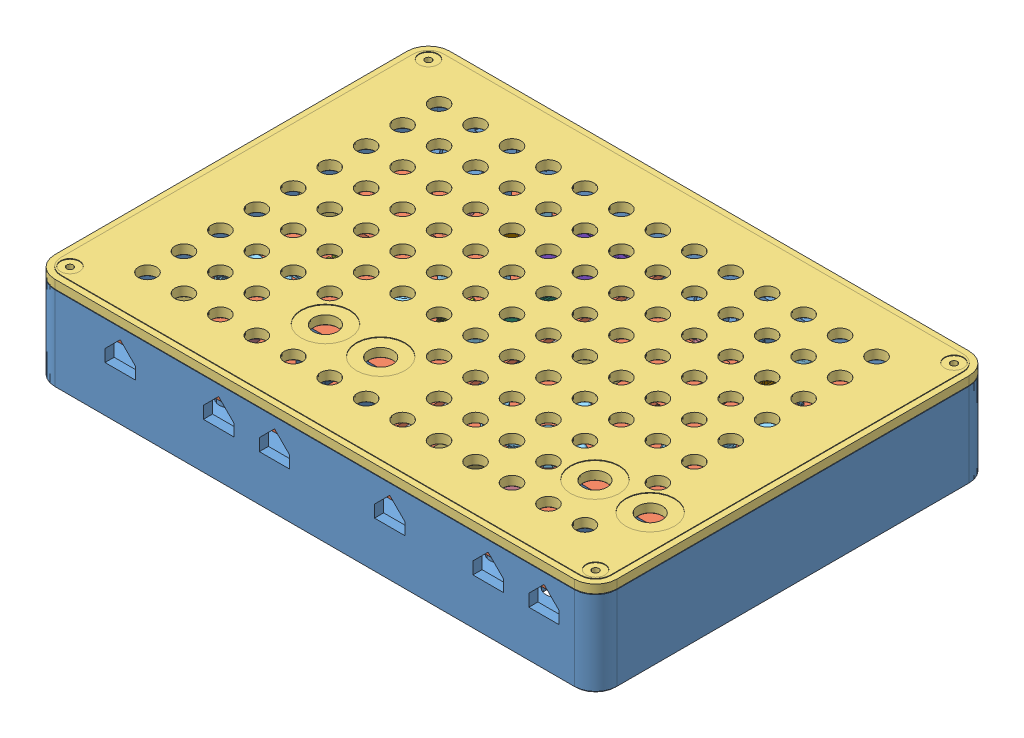
SolidWorks assembly I2SAMP盒子装配, configuration 默认. Lengths in mm.
Overall size (185 31.2 130).
386 component instances, 21 part files, 8 mates.
Components (placement in the parent):
- I2SAMP盒子-1: I2SAMP盒子 [默认] at (-278.4542 45.2933 60) size (185 28 130)
- 3D_I2SInputAmp_1_2024-11-02-1: 3D_I2SInputAmp_1_2024-11-02 [默认] at (-189.7268 58.2933 49.2453) x (0 0 -1) z (0 1 0) size (110.46 78.71 15.8)
  - 3D_I2SInputAmp_1_2024-11-02.step-1: 3D_I2SInputAmp_1_2024-11-02.step [默认] at origin size (110.46 78.71 15.8)
    - 2uP9-L2.step-1: 2uP9-L2.step [默认] at (86.2332 60.9601 1.6001) size (7.42 6.8 3.05)
      - IND-SMD_L7.3-W6.8.step-1: IND-SMD_L7.3-W6.8.step [默认] at origin size (7.42 6.8 3.05)
        - SOLID.step-1: SOLID.step [默认] at origin size (7.42 6.8 3.05)
    - 2uP9-L3.step-1: 2uP9-L3.step [默认] at (86.4872 52.1971 1.6001) size (7.42 6.8 3.05)
      - IND-SMD_L7.3-W6.8.step-1: IND-SMD_L7.3-W6.8.step [默认] at origin size (7.42 6.8 3.05)
        - SOLID.step-1: SOLID.step [默认] at origin size (7.42 6.8 3.05)
    - 2uP9-L4.step-1: 2uP9-L4.step [默认] at (80.8992 44.4501 1.6001) size (7.42 6.8 3.05)
      - IND-SMD_L7.3-W6.8.step-1: IND-SMD_L7.3-W6.8.step [默认] at origin size (7.42 6.8 3.05)
        - SOLID.step-1: SOLID.step [默认] at origin size (7.42 6.8 3.05)
    - 2uP9-L1.step-1: 2uP9-L1.step [默认] at (80.6452 70.3581 1.6001) size (7.42 6.8 3.05)
      - IND-SMD_L7.3-W6.8.step-1: IND-SMD_L7.3-W6.8.step [默认] at origin size (7.42 6.8 3.05)
        - SOLID.step-1: SOLID.step [默认] at origin size (7.42 6.8 3.05)
    - 2uP9-C111.step-1: 2uP9-C111.step [默认] at (64.6431 69.7231 1.6001) size (11.6 10.3 10.21)
      - CAP-SMD_BD10.0-L10.3-W10.3-LS11.0-FD.step-1: CAP-SMD_BD10.0-L10.3-W10.3-LS11.0-FD.step [默认] at origin size (11.6 10.3 10.21)
        - COMPOUND.step-1: COMPOUND.step [默认] at origin size (11.6 10.3 10.21)
    - 2uP9-C108.step-1: 2uP9-C108.step [默认] at (87.8528 41.5212 1.6001) x (-1 0 0) z (0 0 1) size (2 1.3 1.3)
      - C0805.step-1: C0805.step [默认] at origin size (2 1.3 1.3)
        - SOLID-0.step-1: SOLID-0.step [默认] at origin size (2 1.3 1.3)
    - 2uP9-C109.step-1: 2uP9-C109.step [默认] at (92.4562 48.6411 1.6001) x (0 1 0) z (0 0 1) size (2 1.3 1.3)
      - C0805.step-1: C0805.step [默认] at origin size (2 1.3 1.3)
        - SOLID-0.step-1: SOLID-0.step [默认] at origin size (2 1.3 1.3)
    - 2uP9-C110.step-1: 2uP9-C110.step [默认] at (93.2182 62.7381 1.6001) x (0 -1 0) z (0 0 1) size (2 1.3 1.3)
      - C0805.step-1: C0805.step [默认] at origin size (2 1.3 1.3)
        - SOLID-0.step-1: SOLID-0.step [默认] at origin size (2 1.3 1.3)
    - 2uP9-C107.step-1: 2uP9-C107.step [默认] at (88.0112 72.7711 1.6001) size (2 1.3 1.3)
      - C0805.step-1: C0805.step [默认] at origin size (2 1.3 1.3)
        - SOLID-0.step-1: SOLID-0.step [默认] at origin size (2 1.3 1.3)
    - 2uP9-C93.step-1: 2uP9-C93.step [默认] at (35.6871 71.6281 1.6001) size (7.8 6.6 7.75)
      - CAP-SMD_BD6.3-L6.6-W6.6-FD.step-1: CAP-SMD_BD6.3-L6.6-W6.6-FD.step [默认] at origin size (7.8 6.6 7.75)
        - SOLID-1.step-1: SOLID-1.step [默认] at origin size (7.8 6.6 7.75)
    - 2uP9-C94.step-1: 2uP9-C94.step [默认] at (35.6871 63.6271 1.6001) size (7.8 6.6 7.75)
      - CAP-SMD_BD6.3-L6.6-W6.6-FD.step-1: CAP-SMD_BD6.3-L6.6-W6.6-FD.step [默认] at origin size (7.8 6.6 7.75)
        - SOLID-1.step-1: SOLID-1.step [默认] at origin size (7.8 6.6 7.75)
    - 2uP9-C112.step-1: 2uP9-C112.step [默认] at (48.7681 57.7851 1.6001) x (0 1 0) z (0 0 1) size (7.8 6.6 7.75)
      - CAP-SMD_BD6.3-L6.6-W6.6-FD.step-1: CAP-SMD_BD6.3-L6.6-W6.6-FD.step [默认] at origin size (7.8 6.6 7.75)
        - SOLID-1.step-1: SOLID-1.step [默认] at origin size (7.8 6.6 7.75)
    - 2uP9-C113.step-1: 2uP9-C113.step [默认] at (35.4331 45.7201 1.6001) size (7.8 6.6 7.75)
      - CAP-SMD_BD6.3-L6.6-W6.6-FD.step-1: CAP-SMD_BD6.3-L6.6-W6.6-FD.step [默认] at origin size (7.8 6.6 7.75)
        - SOLID-1.step-1: SOLID-1.step [默认] at origin size (7.8 6.6 7.75)
    - 2uP9-C114.step-1: 2uP9-C114.step [默认] at (35.5601 54.3561 1.6001) size (7.8 6.6 7.75)
      - CAP-SMD_BD6.3-L6.6-W6.6-FD.step-1: CAP-SMD_BD6.3-L6.6-W6.6-FD.step [默认] at origin size (7.8 6.6 7.75)
        - SOLID-1.step-1: SOLID-1.step [默认] at origin size (7.8 6.6 7.75)
    - 2uP9-C118.step-1: 2uP9-C118.step [默认] at (51.8161 29.2101 1.6001) x (0 1 0) z (0 0 1) size (7.8 6.6 7.75)
      - CAP-SMD_BD6.3-L6.6-W6.6-FD.step-1: CAP-SMD_BD6.3-L6.6-W6.6-FD.step [默认] at origin size (7.8 6.6 7.75)
        - SOLID-1.step-1: SOLID-1.step [默认] at origin size (7.8 6.6 7.75)
    - 2uP9-C120.step-1: 2uP9-C120.step [默认] at (67.4371 29.4641 1.6001) x (0 1 0) z (0 0 1) size (7.8 6.6 7.75)
      - CAP-SMD_BD6.3-L6.6-W6.6-FD.step-1: CAP-SMD_BD6.3-L6.6-W6.6-FD.step [默认] at origin size (7.8 6.6 7.75)
        - SOLID-1.step-1: SOLID-1.step [默认] at origin size (7.8 6.6 7.75)
    - 2uP9-C124.step-1: 2uP9-C124.step [默认] at (52.5781 8.382 1.6001) x (0 -1 0) z (0 0 1) size (7.8 6.6 7.75)
      - CAP-SMD_BD6.3-L6.6-W6.6-FD.step-1: CAP-SMD_BD6.3-L6.6-W6.6-FD.step [默认] at origin size (7.8 6.6 7.75)
        - SOLID-1.step-1: SOLID-1.step [默认] at origin size (7.8 6.6 7.75)
    - 2uP9-C125.step-1: 2uP9-C125.step [默认] at (73.9141 20.828 1.6001) x (0 1 0) z (0 0 1) size (7.8 6.6 7.75)
      - CAP-SMD_BD6.3-L6.6-W6.6-FD.step-1: CAP-SMD_BD6.3-L6.6-W6.6-FD.step [默认] at origin size (7.8 6.6 7.75)
        - SOLID-1.step-1: SOLID-1.step [默认] at origin size (7.8 6.6 7.75)
    - 2uP9-C51.step-1: 2uP9-C51.step [默认] at (100.9845 34.2354 1.6001) size (7.8 6.6 7.75)
      - CAP-SMD_BD6.3-L6.6-W6.6-FD.step-1: CAP-SMD_BD6.3-L6.6-W6.6-FD.step [默认] at origin size (7.8 6.6 7.75)
        - SOLID-1.step-1: SOLID-1.step [默认] at origin size (7.8 6.6 7.75)
    - 2uP9-RN4.step-1: 2uP9-RN4.step [默认] at (60.9601 44.1961 1.6001) x (0 1 0) z (0 0 1) size (3.2 1.6 0.5)
      - RES-ARRAY-SMD_0603-8P-L3.2-W1.6-BL.step-1: RES-ARRAY-SMD_0603-8P-L3.2-W1.6-BL.step [默认] at origin size (3.2 1.6 0.5)
        - COMPOUND-2.step-1: COMPOUND-2.step [默认] at origin size (3.2 1.6 0.5)
    - 2uP9-RN3.step-1: 2uP9-RN3.step [默认] at (68.9611 44.1961 1.6001) size (3.2 1.6 0.5)
      - RES-ARRAY-SMD_0603-8P-L3.2-W1.6-BL.step-1: RES-ARRAY-SMD_0603-8P-L3.2-W1.6-BL.step [默认] at origin size (3.2 1.6 0.5)
        - COMPOUND-2.step-1: COMPOUND-2.step [默认] at origin size (3.2 1.6 0.5)
    - 2uP9-C52.step-1: 2uP9-C52.step [默认] at (98.8255 28.3934 1.6001) x (0 -1 0) z (0 0 1) size (1.6 0.8 0.8)
      - C0603.step-1: C0603.step [默认] at origin size (1.6 0.8 0.8)
        - SOLID-3.step-1: SOLID-3.step [默认] at origin size (1.6 0.8 0.8)
    - 2uP9-C95.step-1: 2uP9-C95.step [默认] at (57.2771 61.0871 1.6001) size (1.6 0.8 0.8)
      - C0603.step-1: C0603.step [默认] at origin size (1.6 0.8 0.8)
        - SOLID-3.step-1: SOLID-3.step [默认] at origin size (1.6 0.8 0.8)
    - 2uP9-C96.step-1: 2uP9-C96.step [默认] at (73.2791 62.2301 1.6001) size (1.6 0.8 0.8)
      - C0603.step-1: C0603.step [默认] at origin size (1.6 0.8 0.8)
        - SOLID-3.step-1: SOLID-3.step [默认] at origin size (1.6 0.8 0.8)
    - 2uP9-C97.step-1: 2uP9-C97.step [默认] at (56.0071 57.9121 1.6001) x (0 1 0) z (0 0 1) size (1.6 0.8 0.8)
      - C0603.step-1: C0603.step [默认] at origin size (1.6 0.8 0.8)
        - SOLID-3.step-1: SOLID-3.step [默认] at origin size (1.6 0.8 0.8)
    - 2uP9-C98.step-1: 2uP9-C98.step [默认] at (57.9121 57.9121 1.6001) x (0 1 0) z (0 0 1) size (1.6 0.8 0.8)
      - C0603.step-1: C0603.step [默认] at origin size (1.6 0.8 0.8)
        - SOLID-3.step-1: SOLID-3.step [默认] at origin size (1.6 0.8 0.8)
    - 2uP9-C99.step-1: 2uP9-C99.step [默认] at (73.2791 60.431 1.6001) x (-1 0 0) z (0 0 1) size (1.6 0.8 0.8)
      - C0603.step-1: C0603.step [默认] at origin size (1.6 0.8 0.8)
        - SOLID-3.step-1: SOLID-3.step [默认] at origin size (1.6 0.8 0.8)
    - 2uP9-C100.step-1: 2uP9-C100.step [默认] at (73.2791 56.8326 1.6001) x (-1 0 0) z (0 0 1) size (1.6 0.8 0.8)
      - C0603.step-1: C0603.step [默认] at origin size (1.6 0.8 0.8)
        - SOLID-3.step-1: SOLID-3.step [默认] at origin size (1.6 0.8 0.8)
    - 2uP9-C101.step-1: 2uP9-C101.step [默认] at (73.2791 54.9911 1.6001) x (-1 0 0) z (0 0 1) size (1.6 0.8 0.8)
      - C0603.step-1: C0603.step [默认] at origin size (1.6 0.8 0.8)
        - SOLID-3.step-1: SOLID-3.step [默认] at origin size (1.6 0.8 0.8)
    - 2uP9-C102.step-1: 2uP9-C102.step [默认] at (73.2791 51.4351 1.6001) x (-1 0 0) z (0 0 1) size (1.6 0.8 0.8)
      - C0603.step-1: C0603.step [默认] at origin size (1.6 0.8 0.8)
        - SOLID-3.step-1: SOLID-3.step [默认] at origin size (1.6 0.8 0.8)
    - 2uP9-C103.step-1: 2uP9-C103.step [默认] at (57.1501 54.8641 1.6001) x (-1 0 0) z (0 0 1) size (1.6 0.8 0.8)
      - C0603.step-1: C0603.step [默认] at origin size (1.6 0.8 0.8)
        - SOLID-3.step-1: SOLID-3.step [默认] at origin size (1.6 0.8 0.8)
    - 2uP9-C104.step-1: 2uP9-C104.step [默认] at (57.2771 63.1191 1.6001) x (-1 0 0) z (0 0 1) size (1.6 0.8 0.8)
      - C0603.step-1: C0603.step [默认] at origin size (1.6 0.8 0.8)
        - SOLID-3.step-1: SOLID-3.step [默认] at origin size (1.6 0.8 0.8)
    - 2uP9-C105.step-1: 2uP9-C105.step [默认] at (73.2637 58.6372 1.6001) x (-1 0 0) z (0 0 1) size (1.6 0.8 0.8)
      - C0603.step-1: C0603.step [默认] at origin size (1.6 0.8 0.8)
        - SOLID-3.step-1: SOLID-3.step [默认] at origin size (1.6 0.8 0.8)
    - 2uP9-C106.step-1: 2uP9-C106.step [默认] at (73.2791 53.2131 1.6001) x (-1 0 0) z (0 0 1) size (1.6 0.8 0.8)
      - C0603.step-1: C0603.step [默认] at origin size (1.6 0.8 0.8)
        - SOLID-3.step-1: SOLID-3.step [默认] at origin size (1.6 0.8 0.8)
    - 2uP9-C115.step-1: 2uP9-C115.step [默认] at (51.8161 14.986 1.6001) size (1.6 0.8 0.8)
      - C0603.step-1: C0603.step [默认] at origin size (1.6 0.8 0.8)
        - SOLID-3.step-1: SOLID-3.step [默认] at origin size (1.6 0.8 0.8)
    - 2uP9-C116.step-1: 2uP9-C116.step [默认] at (67.5641 17.78 1.6001) x (-1 0 0) z (0 0 1) size (1.6 0.8 0.8)
      - C0603.step-1: C0603.step [默认] at origin size (1.6 0.8 0.8)
        - SOLID-3.step-1: SOLID-3.step [默认] at origin size (1.6 0.8 0.8)
    - 2uP9-C117.step-1: 2uP9-C117.step [默认] at (57.0231 25.1461 1.6001) size (1.6 0.8 0.8)
      - C0603.step-1: C0603.step [默认] at origin size (1.6 0.8 0.8)
        - SOLID-3.step-1: SOLID-3.step [默认] at origin size (1.6 0.8 0.8)
    - 2uP9-C119.step-1: 2uP9-C119.step [默认] at (62.3571 25.1461 1.6001) x (-1 0 0) z (0 0 1) size (1.6 0.8 0.8)
      - C0603.step-1: C0603.step [默认] at origin size (1.6 0.8 0.8)
        - SOLID-3.step-1: SOLID-3.step [默认] at origin size (1.6 0.8 0.8)
    - 2uP9-C121.step-1: 2uP9-C121.step [默认] at (51.8161 22.479 1.6001) x (-1 0 0) z (0 0 1) size (1.6 0.8 0.8)
      - C0603.step-1: C0603.step [默认] at origin size (1.6 0.8 0.8)
        - SOLID-3.step-1: SOLID-3.step [默认] at origin size (1.6 0.8 0.8)
    - 2uP9-C123.step-1: 2uP9-C123.step [默认] at (67.5641 22.86 1.6001) size (1.6 0.8 0.8)
      - C0603.step-1: C0603.step [默认] at origin size (1.6 0.8 0.8)
        - SOLID-3.step-1: SOLID-3.step [默认] at origin size (1.6 0.8 0.8)
    - 2uP9-C126.step-1: 2uP9-C126.step [默认] at (67.5641 20.32 1.6001) x (-1 0 0) z (0 0 1) size (1.6 0.8 0.8)
      - C0603.step-1: C0603.step [默认] at origin size (1.6 0.8 0.8)
        - SOLID-3.step-1: SOLID-3.step [默认] at origin size (1.6 0.8 0.8)
    - 2uP9-C127.step-1: 2uP9-C127.step [默认] at (52.3241 19.685 1.6001) x (0 1 0) z (0 0 1) size (1.6 0.8 0.8)
      - C0603.step-1: C0603.step [默认] at origin size (1.6 0.8 0.8)
        - SOLID-3.step-1: SOLID-3.step [默认] at origin size (1.6 0.8 0.8)
    - 2uP9-C50.step-1: 2uP9-C50.step [默认] at (102.2545 28.3934 1.6001) x (0 1 0) z (0 0 1) size (1.6 0.8 0.8)
      - C0603.step-1: C0603.step [默认] at origin size (1.6 0.8 0.8)
        - SOLID-3.step-1: SOLID-3.step [默认] at origin size (1.6 0.8 0.8)
    - 2uP9-R29.step-1: 2uP9-R29.step [默认] at (13.208 9.652 1.6001) x (0 1 0) z (0 0 1) size (6.3 3.2 0.61)
      - R2512.step-1: R2512.step [默认] at origin size (6.3 3.2 0.61)
        - COMPOUND-4.step-1: COMPOUND-4.step [默认] at origin size (6.3 3.2 0.61)
    - 2uP9-R28.step-1: 2uP9-R28.step [默认] at (13.208 27.9401 1.6001) x (0 1 0) z (0 0 1) size (6.3 3.2 0.61)
      - R2512.step-1: R2512.step [默认] at origin size (6.3 3.2 0.61)
        - COMPOUND-4.step-1: COMPOUND-4.step [默认] at origin size (6.3 3.2 0.61)
    - 2uP9-SETTING0.step-1: 2uP9-SETTING0.step [默认] at (88.2652 35.3061 1.6001) size (7.5 5.9 10.6)
      - CONN-TH_2P-P2.50_HX25003-2A.step-1: CONN-TH_2P-P2.50_HX25003-2A.step [默认] at origin size (7.5 5.9 10.6)
        - COMPOUND-5.step-1: COMPOUND-5.step [默认] at origin size (7.5 5.9 10.6)
    - 2uP9-R35.step-1: 2uP9-R35.step [默认] at (21.7482 9.4159 1.6001) x (-1 0 0) z (0 0 1) size (4.85 9.5 15)
      - RES-ADJ-TH_3P-L10.0-W10.0-P2.50-BL-BS.step-1: RES-ADJ-TH_3P-L10.0-W10.0-P2.50-BL-BS.step [默认] at origin size (4.85 9.5 15)
        - SOLID-6.step-1: SOLID-6.step [默认] at origin size (4.85 9.5 15)
    - 2uP9-R34.step-1: 2uP9-R34.step [默认] at (21.971 27.8131 1.6001) x (-1 0 0) z (0 0 1) size (4.85 9.5 15)
      - RES-ADJ-TH_3P-L10.0-W10.0-P2.50-BL-BS.step-1: RES-ADJ-TH_3P-L10.0-W10.0-P2.50-BL-BS.step [默认] at origin size (4.85 9.5 15)
        - SOLID-6.step-1: SOLID-6.step [默认] at origin size (4.85 9.5 15)
    - 2uP9-U15.step-1: 2uP9-U15.step [默认] at (65.2781 56.2611 1.6001) x (0 -1 0) z (0 0 1) size (11 8.1 1.16)
      - HTSSOP-32_L11.0-W6.1-P0.65-LS8.1-BL-EP-4.step-1: HTSSOP-32_L11.0-W6.1-P0.65-LS8.1-BL-EP-4.step [默认] at origin size (11 8.1 1.16)
        - SOLID-7.step-1: SOLID-7.step [默认] at origin size (11 8.1 1.16)
    - 2uP9-U20.step-1: 2uP9-U20.step [默认] at (22.535 67.3391 1.6001) size (14.23 10.2 4.5)
      - TO-263-3_L8.6-W10.2-P2.54-LS14.4-BR.step-1: TO-263-3_L8.6-W10.2-P2.54-LS14.4-BR.step [默认] at origin size (14.23 10.2 4.5)
        - COMPOUND-8.step-1: COMPOUND-8.step [默认] at origin size (14.23 10.2 4.5)
    - 2uP9-U23.step-1: 2uP9-U23.step [默认] at (20.701 50.1651 1.6001) size (9.92 6.6 2.3)
      - TO-252-2_L6.6-W6.1-P4.57-LS9.9-BR-CW.step-1: TO-252-2_L6.6-W6.1-P4.57-LS9.9-BR-CW.step [默认] at origin size (9.92 6.6 2.3)
        - COMPOUND-9.step-1: COMPOUND-9.step [默认] at origin size (9.92 6.6 2.3)
    - 2uP9-R33.step-1: 2uP9-R33.step [默认] at (96.2855 28.3934 1.6001) x (0 1 0) z (0 0 1) size (1.62 0.81 0.45)
      - R0603.step-1: R0603.step [默认] at origin size (1.62 0.81 0.45)
        - COMPOUND-10.step-1: COMPOUND-10.step [默认] at origin size (1.62 0.81 0.45)
    - 2uP9-R32.step-1: 2uP9-R32.step [默认] at (92.7295 28.5204 1.6001) x (0 1 0) z (0 0 1) size (1.62 0.81 0.45)
      - R0603.step-1: R0603.step [默认] at origin size (1.62 0.81 0.45)
        - COMPOUND-10.step-1: COMPOUND-10.step [默认] at origin size (1.62 0.81 0.45)
    - 2uP9-U14.step-1: 2uP9-U14.step [默认] at (71.7551 7.62 1.6001) x (-1 0 0) z (0 0 1) size (15 5.91 10.4)
      - CONN-TH_5P-P2.50_ZX-XH2.54-5PZZ.step-1: CONN-TH_5P-P2.50_ZX-XH2.54-5PZZ.step [默认] at origin size (15 5.91 10.4)
        - SOLID-11.step-1: SOLID-11.step [默认] at origin size (15 5.91 10.4)
    - 2uP9-U16.step-1: 2uP9-U16.step [默认] at (59.6901 18.796 1.6001) x (0 -1 0) z (0 0 1) size (10.2 7.8 2.2)
      - SSOP-28_L10.2-W5.3-P0.65-LS7.8-BL.step-1: SSOP-28_L10.2-W5.3-P0.65-LS7.8-BL.step [默认] at origin size (10.2 7.8 2.2)
        - SOLID-12.step-1: SOLID-12.step [默认] at origin size (10.2 7.8 2.2)
    - 2uP9-U1.step-1: 2uP9-U1.step [默认] at (93.4915 13.9153 1.6001) x (0 -1 0) z (0 0 1) size (18 25.5 3.12)
      - WIFIM-SMD_ESP32-WROOM-32-N4.step-1: WIFIM-SMD_ESP32-WROOM-32-N4.step [默认] at origin size (18 25.5 3.12)
        - SOLID-13.step-1: SOLID-13.step [默认] at origin size (18 25.5 3.12)
    - 2uP9-U19.step-1: 2uP9-U19.step [默认] at (35.3061 9.779 1.6001) x (0 -1 0) z (0 0 1) size (8.01 14 5.02)
      - XFMR-SMD_L10.5-W8.0-P5.00-LS14.0_ED8-600.step-1: XFMR-SMD_L10.5-W8.0-P5.00-LS14.0_ED8-600.step [默认] at origin size (8.01 14 5.02)
        - COMPOUND-14.step-1: COMPOUND-14.step [默认] at origin size (8.01 14 5.02)
    - 2uP9-U18.step-1: 2uP9-U18.step [默认] at (35.0521 27.9401 1.6001) x (0 -1 0) z (0 0 1) size (8.01 14 5.02)
      - XFMR-SMD_L10.5-W8.0-P5.00-LS14.0_ED8-600.step-1: XFMR-SMD_L10.5-W8.0-P5.00-LS14.0_ED8-600.step [默认] at origin size (8.01 14 5.02)
        - COMPOUND-14.step-1: COMPOUND-14.step [默认] at origin size (8.01 14 5.02)
    - 2uP9-U12.step-1: 2uP9-U12.step [默认] at (3.937 27.8131 1.6001) x (0 -1 0) z (0 0 1) size (10.4 7.7 14.2)
      - CONN-TH_P5.00_KF301-5.0-2P.step-1: CONN-TH_P5.00_KF301-5.0-2P.step [默认] at origin size (10.4 7.7 14.2)
        - COMPOUND-15.step-1: COMPOUND-15.step [默认] at origin size (10.4 7.7 14.2)
    - 2uP9-U13.step-1: 2uP9-U13.step [默认] at (3.937 9.398 1.6001) x (0 -1 0) z (0 0 1) size (10.4 7.7 14.2)
      - CONN-TH_P5.00_KF301-5.0-2P.step-1: CONN-TH_P5.00_KF301-5.0-2P.step [默认] at origin size (10.4 7.7 14.2)
        - COMPOUND-15.step-1: COMPOUND-15.step [默认] at origin size (10.4 7.7 14.2)
    - 2uP9-U21.step-1: 2uP9-U21.step [默认] at (100.8382 65.4051 1.6001) x (0 1 0) z (0 0 1) size (10.4 7.7 14.2)
      - CONN-TH_P5.00_KF301-5.0-2P.step-1: CONN-TH_P5.00_KF301-5.0-2P.step [默认] at origin size (10.4 7.7 14.2)
        - COMPOUND-15.step-1: COMPOUND-15.step [默认] at origin size (10.4 7.7 14.2)
    - 2uP9-U22.step-1: 2uP9-U22.step [默认] at (100.9652 51.8161 1.6001) x (0 1 0) z (0 0 1) size (10.4 7.7 14.2)
      - CONN-TH_P5.00_KF301-5.0-2P.step-1: CONN-TH_P5.00_KF301-5.0-2P.step [默认] at origin size (10.4 7.7 14.2)
        - COMPOUND-15.step-1: COMPOUND-15.step [默认] at origin size (10.4 7.7 14.2)
    - 2uP9-U9.step-1: 2uP9-U9.step [默认] at (4.064 60.1981 1.6001) x (0 -1 0) z (0 0 1) size (10.4 7.7 14.2)
      - CONN-TH_P5.00_KF301-5.0-2P.step-1: CONN-TH_P5.00_KF301-5.0-2P.step [默认] at origin size (10.4 7.7 14.2)
        - COMPOUND-15.step-1: COMPOUND-15.step [默认] at origin size (10.4 7.7 14.2)
    - Board.step-1: Board.step [默认] at origin size (110.46 78.71 1.6)
- 3D_I2SInputAmp_1_2024-11-02-2: 3D_I2SInputAmp_1_2024-11-02 [默认] at (-101.012 58.2933 49.2453) x (0 0 -1) z (0 1 0) size (110.46 78.71 15.8)
  - 3D_I2SInputAmp_1_2024-11-02.step-1: 3D_I2SInputAmp_1_2024-11-02.step [默认] at origin size (110.46 78.71 15.8)
    - 2uP9-L2.step-1: 2uP9-L2.step [默认] at (86.2332 60.9601 1.6001) size (7.42 6.8 3.05)
      - IND-SMD_L7.3-W6.8.step-1: IND-SMD_L7.3-W6.8.step [默认] at origin size (7.42 6.8 3.05)
        - SOLID.step-1: SOLID.step [默认] at origin size (7.42 6.8 3.05)
    - 2uP9-L3.step-1: 2uP9-L3.step [默认] at (86.4872 52.1971 1.6001) size (7.42 6.8 3.05)
      - IND-SMD_L7.3-W6.8.step-1: IND-SMD_L7.3-W6.8.step [默认] at origin size (7.42 6.8 3.05)
        - SOLID.step-1: SOLID.step [默认] at origin size (7.42 6.8 3.05)
    - 2uP9-L4.step-1: 2uP9-L4.step [默认] at (80.8992 44.4501 1.6001) size (7.42 6.8 3.05)
      - IND-SMD_L7.3-W6.8.step-1: IND-SMD_L7.3-W6.8.step [默认] at origin size (7.42 6.8 3.05)
        - SOLID.step-1: SOLID.step [默认] at origin size (7.42 6.8 3.05)
    - 2uP9-L1.step-1: 2uP9-L1.step [默认] at (80.6452 70.3581 1.6001) size (7.42 6.8 3.05)
      - IND-SMD_L7.3-W6.8.step-1: IND-SMD_L7.3-W6.8.step [默认] at origin size (7.42 6.8 3.05)
        - SOLID.step-1: SOLID.step [默认] at origin size (7.42 6.8 3.05)
    - 2uP9-C111.step-1: 2uP9-C111.step [默认] at (64.6431 69.7231 1.6001) size (11.6 10.3 10.21)
      - CAP-SMD_BD10.0-L10.3-W10.3-LS11.0-FD.step-1: CAP-SMD_BD10.0-L10.3-W10.3-LS11.0-FD.step [默认] at origin size (11.6 10.3 10.21)
        - COMPOUND.step-1: COMPOUND.step [默认] at origin size (11.6 10.3 10.21)
    - 2uP9-C108.step-1: 2uP9-C108.step [默认] at (87.8528 41.5212 1.6001) x (-1 0 0) z (0 0 1) size (2 1.3 1.3)
      - C0805.step-1: C0805.step [默认] at origin size (2 1.3 1.3)
        - SOLID-0.step-1: SOLID-0.step [默认] at origin size (2 1.3 1.3)
    - 2uP9-C109.step-1: 2uP9-C109.step [默认] at (92.4562 48.6411 1.6001) x (0 1 0) z (0 0 1) size (2 1.3 1.3)
      - C0805.step-1: C0805.step [默认] at origin size (2 1.3 1.3)
        - SOLID-0.step-1: SOLID-0.step [默认] at origin size (2 1.3 1.3)
    - 2uP9-C110.step-1: 2uP9-C110.step [默认] at (93.2182 62.7381 1.6001) x (0 -1 0) z (0 0 1) size (2 1.3 1.3)
      - C0805.step-1: C0805.step [默认] at origin size (2 1.3 1.3)
        - SOLID-0.step-1: SOLID-0.step [默认] at origin size (2 1.3 1.3)
    - 2uP9-C107.step-1: 2uP9-C107.step [默认] at (88.0112 72.7711 1.6001) size (2 1.3 1.3)
      - C0805.step-1: C0805.step [默认] at origin size (2 1.3 1.3)
        - SOLID-0.step-1: SOLID-0.step [默认] at origin size (2 1.3 1.3)
    - 2uP9-C93.step-1: 2uP9-C93.step [默认] at (35.6871 71.6281 1.6001) size (7.8 6.6 7.75)
      - CAP-SMD_BD6.3-L6.6-W6.6-FD.step-1: CAP-SMD_BD6.3-L6.6-W6.6-FD.step [默认] at origin size (7.8 6.6 7.75)
        - SOLID-1.step-1: SOLID-1.step [默认] at origin size (7.8 6.6 7.75)
    - 2uP9-C94.step-1: 2uP9-C94.step [默认] at (35.6871 63.6271 1.6001) size (7.8 6.6 7.75)
      - CAP-SMD_BD6.3-L6.6-W6.6-FD.step-1: CAP-SMD_BD6.3-L6.6-W6.6-FD.step [默认] at origin size (7.8 6.6 7.75)
        - SOLID-1.step-1: SOLID-1.step [默认] at origin size (7.8 6.6 7.75)
    - 2uP9-C112.step-1: 2uP9-C112.step [默认] at (48.7681 57.7851 1.6001) x (0 1 0) z (0 0 1) size (7.8 6.6 7.75)
      - CAP-SMD_BD6.3-L6.6-W6.6-FD.step-1: CAP-SMD_BD6.3-L6.6-W6.6-FD.step [默认] at origin size (7.8 6.6 7.75)
        - SOLID-1.step-1: SOLID-1.step [默认] at origin size (7.8 6.6 7.75)
    - 2uP9-C113.step-1: 2uP9-C113.step [默认] at (35.4331 45.7201 1.6001) size (7.8 6.6 7.75)
      - CAP-SMD_BD6.3-L6.6-W6.6-FD.step-1: CAP-SMD_BD6.3-L6.6-W6.6-FD.step [默认] at origin size (7.8 6.6 7.75)
        - SOLID-1.step-1: SOLID-1.step [默认] at origin size (7.8 6.6 7.75)
    - 2uP9-C114.step-1: 2uP9-C114.step [默认] at (35.5601 54.3561 1.6001) size (7.8 6.6 7.75)
      - CAP-SMD_BD6.3-L6.6-W6.6-FD.step-1: CAP-SMD_BD6.3-L6.6-W6.6-FD.step [默认] at origin size (7.8 6.6 7.75)
        - SOLID-1.step-1: SOLID-1.step [默认] at origin size (7.8 6.6 7.75)
    - 2uP9-C118.step-1: 2uP9-C118.step [默认] at (51.8161 29.2101 1.6001) x (0 1 0) z (0 0 1) size (7.8 6.6 7.75)
      - CAP-SMD_BD6.3-L6.6-W6.6-FD.step-1: CAP-SMD_BD6.3-L6.6-W6.6-FD.step [默认] at origin size (7.8 6.6 7.75)
        - SOLID-1.step-1: SOLID-1.step [默认] at origin size (7.8 6.6 7.75)
    - 2uP9-C120.step-1: 2uP9-C120.step [默认] at (67.4371 29.4641 1.6001) x (0 1 0) z (0 0 1) size (7.8 6.6 7.75)
      - CAP-SMD_BD6.3-L6.6-W6.6-FD.step-1: CAP-SMD_BD6.3-L6.6-W6.6-FD.step [默认] at origin size (7.8 6.6 7.75)
        - SOLID-1.step-1: SOLID-1.step [默认] at origin size (7.8 6.6 7.75)
    - 2uP9-C124.step-1: 2uP9-C124.step [默认] at (52.5781 8.382 1.6001) x (0 -1 0) z (0 0 1) size (7.8 6.6 7.75)
      - CAP-SMD_BD6.3-L6.6-W6.6-FD.step-1: CAP-SMD_BD6.3-L6.6-W6.6-FD.step [默认] at origin size (7.8 6.6 7.75)
        - SOLID-1.step-1: SOLID-1.step [默认] at origin size (7.8 6.6 7.75)
    - 2uP9-C125.step-1: 2uP9-C125.step [默认] at (73.9141 20.828 1.6001) x (0 1 0) z (0 0 1) size (7.8 6.6 7.75)
      - CAP-SMD_BD6.3-L6.6-W6.6-FD.step-1: CAP-SMD_BD6.3-L6.6-W6.6-FD.step [默认] at origin size (7.8 6.6 7.75)
        - SOLID-1.step-1: SOLID-1.step [默认] at origin size (7.8 6.6 7.75)
    - 2uP9-C51.step-1: 2uP9-C51.step [默认] at (100.9845 34.2354 1.6001) size (7.8 6.6 7.75)
      - CAP-SMD_BD6.3-L6.6-W6.6-FD.step-1: CAP-SMD_BD6.3-L6.6-W6.6-FD.step [默认] at origin size (7.8 6.6 7.75)
        - SOLID-1.step-1: SOLID-1.step [默认] at origin size (7.8 6.6 7.75)
    - 2uP9-RN4.step-1: 2uP9-RN4.step [默认] at (60.9601 44.1961 1.6001) x (0 1 0) z (0 0 1) size (3.2 1.6 0.5)
      - RES-ARRAY-SMD_0603-8P-L3.2-W1.6-BL.step-1: RES-ARRAY-SMD_0603-8P-L3.2-W1.6-BL.step [默认] at origin size (3.2 1.6 0.5)
        - COMPOUND-2.step-1: COMPOUND-2.step [默认] at origin size (3.2 1.6 0.5)
    - 2uP9-RN3.step-1: 2uP9-RN3.step [默认] at (68.9611 44.1961 1.6001) size (3.2 1.6 0.5)
      - RES-ARRAY-SMD_0603-8P-L3.2-W1.6-BL.step-1: RES-ARRAY-SMD_0603-8P-L3.2-W1.6-BL.step [默认] at origin size (3.2 1.6 0.5)
        - COMPOUND-2.step-1: COMPOUND-2.step [默认] at origin size (3.2 1.6 0.5)
    - 2uP9-C52.step-1: 2uP9-C52.step [默认] at (98.8255 28.3934 1.6001) x (0 -1 0) z (0 0 1) size (1.6 0.8 0.8)
      - C0603.step-1: C0603.step [默认] at origin size (1.6 0.8 0.8)
        - SOLID-3.step-1: SOLID-3.step [默认] at origin size (1.6 0.8 0.8)
    - 2uP9-C95.step-1: 2uP9-C95.step [默认] at (57.2771 61.0871 1.6001) size (1.6 0.8 0.8)
      - C0603.step-1: C0603.step [默认] at origin size (1.6 0.8 0.8)
        - SOLID-3.step-1: SOLID-3.step [默认] at origin size (1.6 0.8 0.8)
    - 2uP9-C96.step-1: 2uP9-C96.step [默认] at (73.2791 62.2301 1.6001) size (1.6 0.8 0.8)
      - C0603.step-1: C0603.step [默认] at origin size (1.6 0.8 0.8)
        - SOLID-3.step-1: SOLID-3.step [默认] at origin size (1.6 0.8 0.8)
    - 2uP9-C97.step-1: 2uP9-C97.step [默认] at (56.0071 57.9121 1.6001) x (0 1 0) z (0 0 1) size (1.6 0.8 0.8)
      - C0603.step-1: C0603.step [默认] at origin size (1.6 0.8 0.8)
        - SOLID-3.step-1: SOLID-3.step [默认] at origin size (1.6 0.8 0.8)
    - 2uP9-C98.step-1: 2uP9-C98.step [默认] at (57.9121 57.9121 1.6001) x (0 1 0) z (0 0 1) size (1.6 0.8 0.8)
      - C0603.step-1: C0603.step [默认] at origin size (1.6 0.8 0.8)
        - SOLID-3.step-1: SOLID-3.step [默认] at origin size (1.6 0.8 0.8)
    - 2uP9-C99.step-1: 2uP9-C99.step [默认] at (73.2791 60.431 1.6001) x (-1 0 0) z (0 0 1) size (1.6 0.8 0.8)
      - C0603.step-1: C0603.step [默认] at origin size (1.6 0.8 0.8)
        - SOLID-3.step-1: SOLID-3.step [默认] at origin size (1.6 0.8 0.8)
    - 2uP9-C100.step-1: 2uP9-C100.step [默认] at (73.2791 56.8326 1.6001) x (-1 0 0) z (0 0 1) size (1.6 0.8 0.8)
      - C0603.step-1: C0603.step [默认] at origin size (1.6 0.8 0.8)
        - SOLID-3.step-1: SOLID-3.step [默认] at origin size (1.6 0.8 0.8)
    - 2uP9-C101.step-1: 2uP9-C101.step [默认] at (73.2791 54.9911 1.6001) x (-1 0 0) z (0 0 1) size (1.6 0.8 0.8)
      - C0603.step-1: C0603.step [默认] at origin size (1.6 0.8 0.8)
        - SOLID-3.step-1: SOLID-3.step [默认] at origin size (1.6 0.8 0.8)
    - 2uP9-C102.step-1: 2uP9-C102.step [默认] at (73.2791 51.4351 1.6001) x (-1 0 0) z (0 0 1) size (1.6 0.8 0.8)
      - C0603.step-1: C0603.step [默认] at origin size (1.6 0.8 0.8)
        - SOLID-3.step-1: SOLID-3.step [默认] at origin size (1.6 0.8 0.8)
    - 2uP9-C103.step-1: 2uP9-C103.step [默认] at (57.1501 54.8641 1.6001) x (-1 0 0) z (0 0 1) size (1.6 0.8 0.8)
      - C0603.step-1: C0603.step [默认] at origin size (1.6 0.8 0.8)
        - SOLID-3.step-1: SOLID-3.step [默认] at origin size (1.6 0.8 0.8)
    - 2uP9-C104.step-1: 2uP9-C104.step [默认] at (57.2771 63.1191 1.6001) x (-1 0 0) z (0 0 1) size (1.6 0.8 0.8)
      - C0603.step-1: C0603.step [默认] at origin size (1.6 0.8 0.8)
        - SOLID-3.step-1: SOLID-3.step [默认] at origin size (1.6 0.8 0.8)
    - 2uP9-C105.step-1: 2uP9-C105.step [默认] at (73.2637 58.6372 1.6001) x (-1 0 0) z (0 0 1) size (1.6 0.8 0.8)
      - C0603.step-1: C0603.step [默认] at origin size (1.6 0.8 0.8)
        - SOLID-3.step-1: SOLID-3.step [默认] at origin size (1.6 0.8 0.8)
    - 2uP9-C106.step-1: 2uP9-C106.step [默认] at (73.2791 53.2131 1.6001) x (-1 0 0) z (0 0 1) size (1.6 0.8 0.8)
      - C0603.step-1: C0603.step [默认] at origin size (1.6 0.8 0.8)
        - SOLID-3.step-1: SOLID-3.step [默认] at origin size (1.6 0.8 0.8)
    - 2uP9-C115.step-1: 2uP9-C115.step [默认] at (51.8161 14.986 1.6001) size (1.6 0.8 0.8)
      - C0603.step-1: C0603.step [默认] at origin size (1.6 0.8 0.8)
        - SOLID-3.step-1: SOLID-3.step [默认] at origin size (1.6 0.8 0.8)
    - 2uP9-C116.step-1: 2uP9-C116.step [默认] at (67.5641 17.78 1.6001) x (-1 0 0) z (0 0 1) size (1.6 0.8 0.8)
      - C0603.step-1: C0603.step [默认] at origin size (1.6 0.8 0.8)
        - SOLID-3.step-1: SOLID-3.step [默认] at origin size (1.6 0.8 0.8)
    - 2uP9-C117.step-1: 2uP9-C117.step [默认] at (57.0231 25.1461 1.6001) size (1.6 0.8 0.8)
      - C0603.step-1: C0603.step [默认] at origin size (1.6 0.8 0.8)
        - SOLID-3.step-1: SOLID-3.step [默认] at origin size (1.6 0.8 0.8)
    - 2uP9-C119.step-1: 2uP9-C119.step [默认] at (62.3571 25.1461 1.6001) x (-1 0 0) z (0 0 1) size (1.6 0.8 0.8)
      - C0603.step-1: C0603.step [默认] at origin size (1.6 0.8 0.8)
        - SOLID-3.step-1: SOLID-3.step [默认] at origin size (1.6 0.8 0.8)
    - 2uP9-C121.step-1: 2uP9-C121.step [默认] at (51.8161 22.479 1.6001) x (-1 0 0) z (0 0 1) size (1.6 0.8 0.8)
      - C0603.step-1: C0603.step [默认] at origin size (1.6 0.8 0.8)
        - SOLID-3.step-1: SOLID-3.step [默认] at origin size (1.6 0.8 0.8)
    - 2uP9-C123.step-1: 2uP9-C123.step [默认] at (67.5641 22.86 1.6001) size (1.6 0.8 0.8)
      - C0603.step-1: C0603.step [默认] at origin size (1.6 0.8 0.8)
        - SOLID-3.step-1: SOLID-3.step [默认] at origin size (1.6 0.8 0.8)
    - 2uP9-C126.step-1: 2uP9-C126.step [默认] at (67.5641 20.32 1.6001) x (-1 0 0) z (0 0 1) size (1.6 0.8 0.8)
      - C0603.step-1: C0603.step [默认] at origin size (1.6 0.8 0.8)
        - SOLID-3.step-1: SOLID-3.step [默认] at origin size (1.6 0.8 0.8)
    - 2uP9-C127.step-1: 2uP9-C127.step [默认] at (52.3241 19.685 1.6001) x (0 1 0) z (0 0 1) size (1.6 0.8 0.8)
      - C0603.step-1: C0603.step [默认] at origin size (1.6 0.8 0.8)
        - SOLID-3.step-1: SOLID-3.step [默认] at origin size (1.6 0.8 0.8)
    - 2uP9-C50.step-1: 2uP9-C50.step [默认] at (102.2545 28.3934 1.6001) x (0 1 0) z (0 0 1) size (1.6 0.8 0.8)
      - C0603.step-1: C0603.step [默认] at origin size (1.6 0.8 0.8)
        - SOLID-3.step-1: SOLID-3.step [默认] at origin size (1.6 0.8 0.8)
    - 2uP9-R29.step-1: 2uP9-R29.step [默认] at (13.208 9.652 1.6001) x (0 1 0) z (0 0 1) size (6.3 3.2 0.61)
      - R2512.step-1: R2512.step [默认] at origin size (6.3 3.2 0.61)
        - COMPOUND-4.step-1: COMPOUND-4.step [默认] at origin size (6.3 3.2 0.61)
    - 2uP9-R28.step-1: 2uP9-R28.step [默认] at (13.208 27.9401 1.6001) x (0 1 0) z (0 0 1) size (6.3 3.2 0.61)
      - R2512.step-1: R2512.step [默认] at origin size (6.3 3.2 0.61)
        - COMPOUND-4.step-1: COMPOUND-4.step [默认] at origin size (6.3 3.2 0.61)
    - 2uP9-SETTING0.step-1: 2uP9-SETTING0.step [默认] at (88.2652 35.3061 1.6001) size (7.5 5.9 10.6)
      - CONN-TH_2P-P2.50_HX25003-2A.step-1: CONN-TH_2P-P2.50_HX25003-2A.step [默认] at origin size (7.5 5.9 10.6)
        - COMPOUND-5.step-1: COMPOUND-5.step [默认] at origin size (7.5 5.9 10.6)
    - 2uP9-R35.step-1: 2uP9-R35.step [默认] at (21.7482 9.4159 1.6001) x (-1 0 0) z (0 0 1) size (4.85 9.5 15)
      - RES-ADJ-TH_3P-L10.0-W10.0-P2.50-BL-BS.step-1: RES-ADJ-TH_3P-L10.0-W10.0-P2.50-BL-BS.step [默认] at origin size (4.85 9.5 15)
        - SOLID-6.step-1: SOLID-6.step [默认] at origin size (4.85 9.5 15)
    - 2uP9-R34.step-1: 2uP9-R34.step [默认] at (21.971 27.8131 1.6001) x (-1 0 0) z (0 0 1) size (4.85 9.5 15)
      - RES-ADJ-TH_3P-L10.0-W10.0-P2.50-BL-BS.step-1: RES-ADJ-TH_3P-L10.0-W10.0-P2.50-BL-BS.step [默认] at origin size (4.85 9.5 15)
        - SOLID-6.step-1: SOLID-6.step [默认] at origin size (4.85 9.5 15)
    - 2uP9-U15.step-1: 2uP9-U15.step [默认] at (65.2781 56.2611 1.6001) x (0 -1 0) z (0 0 1) size (11 8.1 1.16)
      - HTSSOP-32_L11.0-W6.1-P0.65-LS8.1-BL-EP-4.step-1: HTSSOP-32_L11.0-W6.1-P0.65-LS8.1-BL-EP-4.step [默认] at origin size (11 8.1 1.16)
        - SOLID-7.step-1: SOLID-7.step [默认] at origin size (11 8.1 1.16)
    - 2uP9-U20.step-1: 2uP9-U20.step [默认] at (22.535 67.3391 1.6001) size (14.23 10.2 4.5)
      - TO-263-3_L8.6-W10.2-P2.54-LS14.4-BR.step-1: TO-263-3_L8.6-W10.2-P2.54-LS14.4-BR.step [默认] at origin size (14.23 10.2 4.5)
        - COMPOUND-8.step-1: COMPOUND-8.step [默认] at origin size (14.23 10.2 4.5)
    - 2uP9-U23.step-1: 2uP9-U23.step [默认] at (20.701 50.1651 1.6001) size (9.92 6.6 2.3)
      - TO-252-2_L6.6-W6.1-P4.57-LS9.9-BR-CW.step-1: TO-252-2_L6.6-W6.1-P4.57-LS9.9-BR-CW.step [默认] at origin size (9.92 6.6 2.3)
        - COMPOUND-9.step-1: COMPOUND-9.step [默认] at origin size (9.92 6.6 2.3)
    - 2uP9-R33.step-1: 2uP9-R33.step [默认] at (96.2855 28.3934 1.6001) x (0 1 0) z (0 0 1) size (1.62 0.81 0.45)
      - R0603.step-1: R0603.step [默认] at origin size (1.62 0.81 0.45)
        - COMPOUND-10.step-1: COMPOUND-10.step [默认] at origin size (1.62 0.81 0.45)
    - 2uP9-R32.step-1: 2uP9-R32.step [默认] at (92.7295 28.5204 1.6001) x (0 1 0) z (0 0 1) size (1.62 0.81 0.45)
      - R0603.step-1: R0603.step [默认] at origin size (1.62 0.81 0.45)
        - COMPOUND-10.step-1: COMPOUND-10.step [默认] at origin size (1.62 0.81 0.45)
    - 2uP9-U14.step-1: 2uP9-U14.step [默认] at (71.7551 7.62 1.6001) x (-1 0 0) z (0 0 1) size (15 5.91 10.4)
      - CONN-TH_5P-P2.50_ZX-XH2.54-5PZZ.step-1: CONN-TH_5P-P2.50_ZX-XH2.54-5PZZ.step [默认] at origin size (15 5.91 10.4)
        - SOLID-11.step-1: SOLID-11.step [默认] at origin size (15 5.91 10.4)
    - 2uP9-U16.step-1: 2uP9-U16.step [默认] at (59.6901 18.796 1.6001) x (0 -1 0) z (0 0 1) size (10.2 7.8 2.2)
      - SSOP-28_L10.2-W5.3-P0.65-LS7.8-BL.step-1: SSOP-28_L10.2-W5.3-P0.65-LS7.8-BL.step [默认] at origin size (10.2 7.8 2.2)
        - SOLID-12.step-1: SOLID-12.step [默认] at origin size (10.2 7.8 2.2)
    - 2uP9-U1.step-1: 2uP9-U1.step [默认] at (93.4915 13.9153 1.6001) x (0 -1 0) z (0 0 1) size (18 25.5 3.12)
      - WIFIM-SMD_ESP32-WROOM-32-N4.step-1: WIFIM-SMD_ESP32-WROOM-32-N4.step [默认] at origin size (18 25.5 3.12)
        - SOLID-13.step-1: SOLID-13.step [默认] at origin size (18 25.5 3.12)
    - 2uP9-U19.step-1: 2uP9-U19.step [默认] at (35.3061 9.779 1.6001) x (0 -1 0) z (0 0 1) size (8.01 14 5.02)
      - XFMR-SMD_L10.5-W8.0-P5.00-LS14.0_ED8-600.step-1: XFMR-SMD_L10.5-W8.0-P5.00-LS14.0_ED8-600.step [默认] at origin size (8.01 14 5.02)
        - COMPOUND-14.step-1: COMPOUND-14.step [默认] at origin size (8.01 14 5.02)
    - 2uP9-U18.step-1: 2uP9-U18.step [默认] at (35.0521 27.9401 1.6001) x (0 -1 0) z (0 0 1) size (8.01 14 5.02)
      - XFMR-SMD_L10.5-W8.0-P5.00-LS14.0_ED8-600.step-1: XFMR-SMD_L10.5-W8.0-P5.00-LS14.0_ED8-600.step [默认] at origin size (8.01 14 5.02)
        - COMPOUND-14.step-1: COMPOUND-14.step [默认] at origin size (8.01 14 5.02)
    - 2uP9-U12.step-1: 2uP9-U12.step [默认] at (3.937 27.8131 1.6001) x (0 -1 0) z (0 0 1) size (10.4 7.7 14.2)
      - CONN-TH_P5.00_KF301-5.0-2P.step-1: CONN-TH_P5.00_KF301-5.0-2P.step [默认] at origin size (10.4 7.7 14.2)
        - COMPOUND-15.step-1: COMPOUND-15.step [默认] at origin size (10.4 7.7 14.2)
    - 2uP9-U13.step-1: 2uP9-U13.step [默认] at (3.937 9.398 1.6001) x (0 -1 0) z (0 0 1) size (10.4 7.7 14.2)
      - CONN-TH_P5.00_KF301-5.0-2P.step-1: CONN-TH_P5.00_KF301-5.0-2P.step [默认] at origin size (10.4 7.7 14.2)
        - COMPOUND-15.step-1: COMPOUND-15.step [默认] at origin size (10.4 7.7 14.2)
    - 2uP9-U21.step-1: 2uP9-U21.step [默认] at (100.8382 65.4051 1.6001) x (0 1 0) z (0 0 1) size (10.4 7.7 14.2)
      - CONN-TH_P5.00_KF301-5.0-2P.step-1: CONN-TH_P5.00_KF301-5.0-2P.step [默认] at origin size (10.4 7.7 14.2)
        - COMPOUND-15.step-1: COMPOUND-15.step [默认] at origin size (10.4 7.7 14.2)
    - 2uP9-U22.step-1: 2uP9-U22.step [默认] at (100.9652 51.8161 1.6001) x (0 1 0) z (0 0 1) size (10.4 7.7 14.2)
      - CONN-TH_P5.00_KF301-5.0-2P.step-1: CONN-TH_P5.00_KF301-5.0-2P.step [默认] at origin size (10.4 7.7 14.2)
        - COMPOUND-15.step-1: COMPOUND-15.step [默认] at origin size (10.4 7.7 14.2)
    - 2uP9-U9.step-1: 2uP9-U9.step [默认] at (4.064 60.1981 1.6001) x (0 -1 0) z (0 0 1) size (10.4 7.7 14.2)
      - CONN-TH_P5.00_KF301-5.0-2P.step-1: CONN-TH_P5.00_KF301-5.0-2P.step [默认] at origin size (10.4 7.7 14.2)
        - COMPOUND-15.step-1: COMPOUND-15.step [默认] at origin size (10.4 7.7 14.2)
    - Board.step-1: Board.step [默认] at origin size (110.46 78.71 1.6)
- I2SAMP盖子-1: I2SAMP盖子 [默认] at (-93.4542 73.2933 60) x (0 0 -1) z (1 0 0) size (130 3.2 185)
Mates (geometry in assembly coordinates):
- 距离1: distance = 10 mm anti-aligned: plane of I2SAMP盒子-1 through (-278.4542 48.2933 60) normal (0 1 0); plane of 3D_I2SInputAmp_1_2024-11-02-1/3D_I2SInputAmp_1_2024-11-02.step-1/Board.step-1 through (-229.0968 58.2933 -5.7458) normal (0 -1 0)
- 距离2: distance = 10 mm aligned: plane of 3D_I2SInputAmp_1_2024-11-02-1/3D_I2SInputAmp_1_2024-11-02.step-1/Board.step-1 through (-268.4542 58.2933 49.4866) normal (-1 0 0); plane of I2SAMP盒子-1 through (-278.4542 48.2933 60) normal (-1 0 0)
- 重合3: coincident aligned: plane of 3D_I2SInputAmp_1_2024-11-02-1/3D_I2SInputAmp_1_2024-11-02.step-1/Board.step-1 through (-229.0968 59.8933 -5.7458) normal (0 1 0); plane of 3D_I2SInputAmp_1_2024-11-02-2/3D_I2SInputAmp_1_2024-11-02.step-1/Board.step-1 through (-140.3821 59.8933 -5.7458) normal (0 1 0)
- 重合4: coincident aligned: plane of 3D_I2SInputAmp_1_2024-11-02-1/3D_I2SInputAmp_1_2024-11-02.step-1/Board.step-1 through (-268.4542 58.2933 -60.9782) normal (0 0 -1); plane of 3D_I2SInputAmp_1_2024-11-02-2/3D_I2SInputAmp_1_2024-11-02.step-1/Board.step-1 through (-179.7395 58.2933 -60.9782) normal (0 0 -1)
- 距离3: distance = 10 mm anti-aligned: plane of 3D_I2SInputAmp_1_2024-11-02-1/3D_I2SInputAmp_1_2024-11-02.step-1/Board.step-1 through (-189.7395 58.2933 -60.9782) normal (1 0 0); plane of 3D_I2SInputAmp_1_2024-11-02-2/3D_I2SInputAmp_1_2024-11-02.step-1/Board.step-1 through (-179.7395 58.2933 49.4866) normal (-1 0 0)
- 重合6: coincident anti-aligned: plane of I2SAMP盒子-1 through (-278.4542 73.2933 60) normal (0 1 0); plane of I2SAMP盖子-1 through (-93.4542 73.2933 60) normal (0 -1 0)
- 同心1: concentric aligned: cylinder of I2SAMP盒子-1 through (-272.4542 63.2933 54) axis (0 1 0) radius 0.9; cylinder of I2SAMP盖子-1 through (-272.4542 73.2933 54) axis (0 1 0) radius 1.1
- 同心2: concentric aligned: circle of I2SAMP盒子-1; cylinder of I2SAMP盖子-1 through (-99.4542 73.2933 -64) axis (0 1 0) radius 1.1
